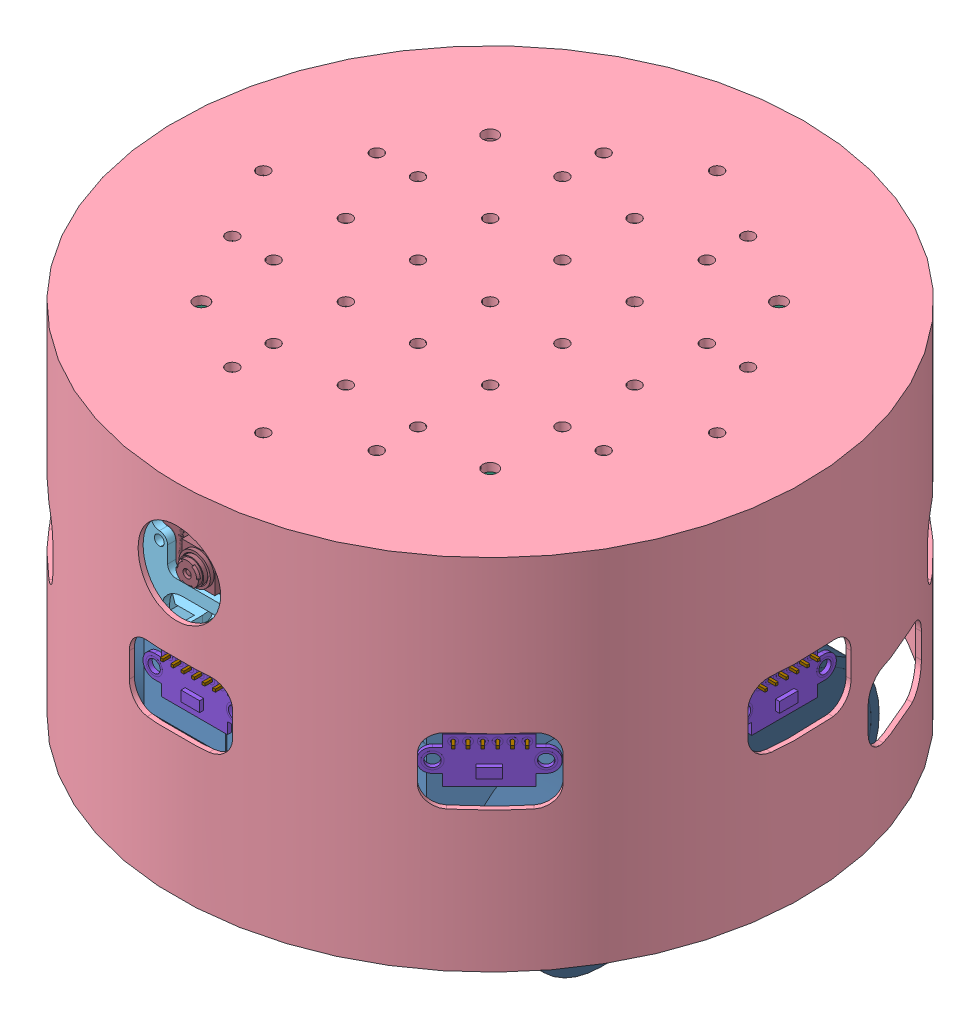
SolidWorks assembly affective_mobile_platform_ver_3, configuration Default. Lengths in mm. (continued)
Components (placement in the parent): (continued)
- outside_case-1: outside_case [Default] at (56.0336 131.8592 98.8354) size (152 87 152)
- 12x1_male_header_pin_AP203-2: 12x1_male_header_pin_AP203 [Default] at (105.1021 111.9373 83.4854) size (2.53 11.54 50.8)
  - 12x1_male_header_pin_AP203.STEP-3: 12x1_male_header_pin_AP203.STEP [Default] at origin size (2.53 11.54 30.48)
    - pin_Predeterminado.STEP-1: pin_Predeterminado.STEP [Default] at (-1.1265 -5.218 11.222) size (0.64 11.54 0.64)
    - pin_body_Predeterminado.STEP-1: pin_body_Predeterminado.STEP [Default] at (-2.0646 3.322 12.8973) x (1 0 0) z (0 -1 0) size (2.53 30.48 2.54)
    - pin_Predeterminado.STEP-2: pin_Predeterminado.STEP [Default] at (-1.1265 -5.218 13.762) size (0.64 11.54 0.64)
    - pin_Predeterminado.STEP-3: pin_Predeterminado.STEP [Default] at (-1.1265 -5.218 16.302) size (0.64 11.54 0.64)
    - pin_Predeterminado.STEP-4: pin_Predeterminado.STEP [Default] at (-1.1265 -5.218 18.842) size (0.64 11.54 0.64)
    - pin_Predeterminado.STEP-5: pin_Predeterminado.STEP [Default] at (-1.1265 -5.218 21.382) size (0.64 11.54 0.64)
    - pin_Predeterminado.STEP-6: pin_Predeterminado.STEP [Default] at (-1.1265 -5.218 23.922) size (0.64 11.54 0.64)
    - pin_Predeterminado.STEP-7: pin_Predeterminado.STEP [Default] at (-1.1265 -5.218 26.462) size (0.64 11.54 0.64)
    - pin_Predeterminado.STEP-8: pin_Predeterminado.STEP [Default] at (-1.1265 -5.218 29.002) size (0.64 11.54 0.64)
    - pin_Predeterminado.STEP-9: pin_Predeterminado.STEP [Default] at (-1.1265 -5.218 31.542) size (0.64 11.54 0.64)
    - pin_Predeterminado.STEP-10: pin_Predeterminado.STEP [Default] at (-1.1265 -5.218 34.082) size (0.64 11.54 0.64)
    - pin_Predeterminado.STEP-11: pin_Predeterminado.STEP [Default] at (-1.1265 -5.218 36.622) size (0.64 11.54 0.64)
    - pin_Predeterminado.STEP-12: pin_Predeterminado.STEP [Default] at (-1.1265 -5.218 39.162) size (0.64 11.54 0.64)
  - 12x1_male_header_pin_AP203.STEP-2: 12x1_male_header_pin_AP203.STEP [Default] at (0 0 -20.32) size (2.53 11.54 30.48)
    - pin_Predeterminado.STEP-1: pin_Predeterminado.STEP [Default] at (-1.1265 -5.218 11.222) size (0.64 11.54 0.64)
    - pin_body_Predeterminado.STEP-1: pin_body_Predeterminado.STEP [Default] at (-2.0646 3.322 12.8973) x (1 0 0) z (0 -1 0) size (2.53 30.48 2.54)
    - pin_Predeterminado.STEP-2: pin_Predeterminado.STEP [Default] at (-1.1265 -5.218 13.762) size (0.64 11.54 0.64)
    - pin_Predeterminado.STEP-3: pin_Predeterminado.STEP [Default] at (-1.1265 -5.218 16.302) size (0.64 11.54 0.64)
    - pin_Predeterminado.STEP-4: pin_Predeterminado.STEP [Default] at (-1.1265 -5.218 18.842) size (0.64 11.54 0.64)
    - pin_Predeterminado.STEP-5: pin_Predeterminado.STEP [Default] at (-1.1265 -5.218 21.382) size (0.64 11.54 0.64)
    - pin_Predeterminado.STEP-6: pin_Predeterminado.STEP [Default] at (-1.1265 -5.218 23.922) size (0.64 11.54 0.64)
    - pin_Predeterminado.STEP-7: pin_Predeterminado.STEP [Default] at (-1.1265 -5.218 26.462) size (0.64 11.54 0.64)
    - pin_Predeterminado.STEP-8: pin_Predeterminado.STEP [Default] at (-1.1265 -5.218 29.002) size (0.64 11.54 0.64)
    - pin_Predeterminado.STEP-9: pin_Predeterminado.STEP [Default] at (-1.1265 -5.218 31.542) size (0.64 11.54 0.64)
    - pin_Predeterminado.STEP-10: pin_Predeterminado.STEP [Default] at (-1.1265 -5.218 34.082) size (0.64 11.54 0.64)
    - pin_Predeterminado.STEP-11: pin_Predeterminado.STEP [Default] at (-1.1265 -5.218 36.622) size (0.64 11.54 0.64)
    - pin_Predeterminado.STEP-12: pin_Predeterminado.STEP [Default] at (-1.1265 -5.218 39.162) size (0.64 11.54 0.64)
- 13x2_female_header^affective_mobile_platform_ver_3-2: 13x2_female_header^affective_mobile_platform_ver_3 [Default] at (128.2122 91.0473 108.7584) x (0 0 1) z (0 1 0) size (50.8 2.5 18) (virtual)
  - Body_Varsay_lan.STEP^13x2_female_header_affective_mobile_platform_ver_3-2: Body_Varsay_lan.STEP^13x2_female_header_affective_mobile_platform_ver_3 [Default] at (33.296 -42.1751 13.1719) size (33.02 2.5 8.5) (virtual)
  - pin_Varsay_lan.STEP^13x2_female_header_affective_mobile_platform_ver_3-28: pin_Varsay_lan.STEP^13x2_female_header_affective_mobile_platform_ver_3 [Default] at (22.3287 -23.5891 -26.7452) x (1 0 0) z (0 -1 0) size (2 16.29 0.4) (virtual)
  - pin_Varsay_lan.STEP^13x2_female_header_affective_mobile_platform_ver_3-30: pin_Varsay_lan.STEP^13x2_female_header_affective_mobile_platform_ver_3 [Default] at (24.8687 -23.5891 -26.7452) x (1 0 0) z (0 -1 0) size (2 16.29 0.4) (virtual)
  - pin_Varsay_lan.STEP^13x2_female_header_affective_mobile_platform_ver_3-32: pin_Varsay_lan.STEP^13x2_female_header_affective_mobile_platform_ver_3 [Default] at (27.4087 -23.5891 -26.7452) x (1 0 0) z (0 -1 0) size (2 16.29 0.4) (virtual)
  - pin_Varsay_lan.STEP^13x2_female_header_affective_mobile_platform_ver_3-34: pin_Varsay_lan.STEP^13x2_female_header_affective_mobile_platform_ver_3 [Default] at (29.9487 -23.5891 -26.7452) x (1 0 0) z (0 -1 0) size (2 16.29 0.4) (virtual)
  - pin_Varsay_lan.STEP^13x2_female_header_affective_mobile_platform_ver_3-36: pin_Varsay_lan.STEP^13x2_female_header_affective_mobile_platform_ver_3 [Default] at (32.4887 -23.5891 -26.7452) x (1 0 0) z (0 -1 0) size (2 16.29 0.4) (virtual)
  - pin_Varsay_lan.STEP^13x2_female_header_affective_mobile_platform_ver_3-38: pin_Varsay_lan.STEP^13x2_female_header_affective_mobile_platform_ver_3 [Default] at (35.0287 -23.5891 -26.7452) x (1 0 0) z (0 -1 0) size (2 16.29 0.4) (virtual)
  - pin_Varsay_lan.STEP^13x2_female_header_affective_mobile_platform_ver_3-40: pin_Varsay_lan.STEP^13x2_female_header_affective_mobile_platform_ver_3 [Default] at (37.5687 -23.5891 -26.7452) x (1 0 0) z (0 -1 0) size (2 16.29 0.4) (virtual)
  - pin_Varsay_lan.STEP^13x2_female_header_affective_mobile_platform_ver_3-42: pin_Varsay_lan.STEP^13x2_female_header_affective_mobile_platform_ver_3 [Default] at (40.1087 -23.5891 -26.7452) x (1 0 0) z (0 -1 0) size (2 16.29 0.4) (virtual)
  - pin_Varsay_lan.STEP^13x2_female_header_affective_mobile_platform_ver_3-44: pin_Varsay_lan.STEP^13x2_female_header_affective_mobile_platform_ver_3 [Default] at (42.6487 -23.5891 -26.7452) x (1 0 0) z (0 -1 0) size (2 16.29 0.4) (virtual)
  - pin_Varsay_lan.STEP^13x2_female_header_affective_mobile_platform_ver_3-46: pin_Varsay_lan.STEP^13x2_female_header_affective_mobile_platform_ver_3 [Default] at (45.1887 -23.5891 -26.7452) x (1 0 0) z (0 -1 0) size (2 16.29 0.4) (virtual)
  - pin_Varsay_lan.STEP^13x2_female_header_affective_mobile_platform_ver_3-48: pin_Varsay_lan.STEP^13x2_female_header_affective_mobile_platform_ver_3 [Default] at (47.7287 -23.5891 -26.7452) x (1 0 0) z (0 -1 0) size (2 16.29 0.4) (virtual)
  - pin_Varsay_lan.STEP^13x2_female_header_affective_mobile_platform_ver_3-50: pin_Varsay_lan.STEP^13x2_female_header_affective_mobile_platform_ver_3 [Default] at (50.2687 -23.5891 -26.7452) x (1 0 0) z (0 -1 0) size (2 16.29 0.4) (virtual)
  - pin_Varsay_lan.STEP^13x2_female_header_affective_mobile_platform_ver_3-52: pin_Varsay_lan.STEP^13x2_female_header_affective_mobile_platform_ver_3 [Default] at (52.8087 -23.5891 -26.7452) x (1 0 0) z (0 -1 0) size (2 16.29 0.4) (virtual)
  - Body_Varsay_lan.STEP^13x2_female_header_affective_mobile_platform_ver_3-3: Body_Varsay_lan.STEP^13x2_female_header_affective_mobile_platform_ver_3 [Default] at (51.076 -42.1751 13.1719) size (33.02 2.5 8.5) (virtual)
  - pin_Varsay_lan.STEP^13x2_female_header_affective_mobile_platform_ver_3-53: pin_Varsay_lan.STEP^13x2_female_header_affective_mobile_platform_ver_3 [Default] at (55.3487 -23.5891 -26.7452) x (1 0 0) z (0 -1 0) size (2 16.29 0.4) (virtual)
  - pin_Varsay_lan.STEP^13x2_female_header_affective_mobile_platform_ver_3-54: pin_Varsay_lan.STEP^13x2_female_header_affective_mobile_platform_ver_3 [Default] at (57.8887 -23.5891 -26.7452) x (1 0 0) z (0 -1 0) size (2 16.29 0.4) (virtual)
  - pin_Varsay_lan.STEP^13x2_female_header_affective_mobile_platform_ver_3-55: pin_Varsay_lan.STEP^13x2_female_header_affective_mobile_platform_ver_3 [Default] at (60.4287 -23.5891 -26.7452) x (1 0 0) z (0 -1 0) size (2 16.29 0.4) (virtual)
  - pin_Varsay_lan.STEP^13x2_female_header_affective_mobile_platform_ver_3-56: pin_Varsay_lan.STEP^13x2_female_header_affective_mobile_platform_ver_3 [Default] at (62.9687 -23.5891 -26.7452) x (1 0 0) z (0 -1 0) size (2 16.29 0.4) (virtual)
  - pin_Varsay_lan.STEP^13x2_female_header_affective_mobile_platform_ver_3-57: pin_Varsay_lan.STEP^13x2_female_header_affective_mobile_platform_ver_3 [Default] at (70.5887 -23.5891 -26.7452) x (1 0 0) z (0 -1 0) size (2 16.29 0.4) (virtual)
  - pin_Varsay_lan.STEP^13x2_female_header_affective_mobile_platform_ver_3-58: pin_Varsay_lan.STEP^13x2_female_header_affective_mobile_platform_ver_3 [Default] at (68.0487 -23.5891 -26.7452) x (1 0 0) z (0 -1 0) size (2 16.29 0.4) (virtual)
  - pin_Varsay_lan.STEP^13x2_female_header_affective_mobile_platform_ver_3-61: pin_Varsay_lan.STEP^13x2_female_header_affective_mobile_platform_ver_3 [Default] at (65.5087 -23.5891 -26.7452) x (1 0 0) z (0 -1 0) size (2 16.29 0.4) (virtual)
- pi_cam_holder-1: pi_cam_holder [Default] at (56.0336 90.9064 152.5354) size (63.18 39 21.14)
Mates (geometry in assembly coordinates):
- Coincident1: coincident anti-aligned: plane of main_case_v02-1 through (23.7836 61.1064 146.5354) normal (0 1 0); plane of power_bank-1 through (23.7836 62.6064 146.5354) normal (0 -1 0)
- Coincident2: coincident anti-aligned: plane of main_case-1 through (56.0336 74.2064 146.5354) normal (0 0 -1); plane of power_bank-1 through (56.0336 74.1064 146.5354) normal (0 0 1)
- Width1: width aligned: plane of power_bank-1 through (23.7836 62.6064 146.5354) normal (-1 0 0); plane of power_bank-1 through (88.2836 62.6064 146.5354) normal (1 0 0); plane of main_case-1 through (88.2836 59.1064 146.5354) normal (-1 0 0); plane of main_case-1 through (23.7836 89.3064 146.5354) normal (1 0 0)
- Coincident9: coincident anti-aligned: plane of main_case-1 through (56.0336 74.2064 74.8354) normal (0 0 1); plane of motor_holder-1 through (56.0336 51.1064 74.8354) normal (0 0 -1)
- Coincident10: coincident anti-aligned: plane of main_case-1 through (56.0336 74.2064 51.1354) normal (1 0 0); plane of motor_holder-1 through (56.0336 51.1064 74.8354) normal (-1 0 0)
- Coincident17: coincident aligned: plane of main_case-1 through (94.0836 56.1064 115.3354) normal (1 0 0); plane of wheel_holder-1 through (94.0836 50.1064 122.8354) normal (1 0 0)
- Coincident18: coincident aligned: plane of main_case-1 through (56.0336 74.2064 122.8354) normal (0 0 1); plane of wheel_holder-1 through (74.0836 50.1064 122.8354) normal (0 0 1)
- Concentric1: concentric anti-aligned: cylinder of main_case-1 through (29.5836 56.1064 112.3354) axis (0 -1 0) radius 1.6; cylinder of wheel_holder-2 through (29.5836 51.1064 112.3354) axis (0 1 0) radius 1.6
- Concentric2: concentric anti-aligned: cylinder of main_case-1 through (29.5836 56.1064 133.3354) axis (0 -1 0) radius 1.6; cylinder of wheel_holder-2 through (29.5836 51.1064 133.3354) axis (0 1 0) radius 1.6
- Coincident21: coincident anti-aligned: plane of main_case-1 through (56.0336 56.1064 51.1354) normal (0 -1 0); plane of wheel_holder-1 through (94.0836 56.1064 130.3354) normal (0 1 0)
- Coincident22: coincident anti-aligned: plane of main_case-1 through (56.0336 56.1064 51.1354) normal (0 -1 0); plane of wheel_holder-2 through (17.9836 56.1064 115.3354) normal (0 1 0)
- Coincident23: coincident anti-aligned: plane of main_case-1 through (56.0336 56.1064 51.1354) normal (0 -1 0); plane of motor_holder-1 through (21.7836 56.1064 82.8354) normal (0 1 0)
- Width2: width anti-aligned: plane of power_bank-2 through (56.0336 72.6064 51.0354) normal (0 0 -1); plane of main_case-1 through (56.0336 72.6064 146.6354) normal (0 0 1); plane of power_bank-2 through (56.0336 74.2064 51.1354) normal (0 0 1); plane of main_case-1 through (56.0336 74.2064 146.5354) normal (0 0 -1)
- Width3: width aligned: plane of power_bank-2 through (23.7836 61.1064 51.0354) normal (-1 0 0); plane of main_case-1 through (88.2836 61.1064 51.0354) normal (1 0 0); plane of power_bank-2 through (88.2836 59.1064 146.5354) normal (-1 0 0); plane of main_case-1 through (23.7836 89.3064 146.5354) normal (1 0 0)
- InPlace1: in place: plane of main_case-1 through (21.7836 85.8064 146.5354) normal (0 1 0); plane of ? through (0 85.8064 0) normal (0 1 0); moOrthogonalPlaneRef_w of main_case-1 through (21.7836 85.8064 146.5354) normal (0 1 0); plane of ? through (0 85.8064 0) normal (0 0 -1); plane of main_case-1 through (21.7836 85.8064 146.5354) normal (0 1 0); plane of ? through (0 85.8064 0) normal (1 0 0); plane of main_case-1 through (21.7836 89.3064 146.5354) normal (0 1 0); unknown of ?
- Coincident25: coincident aligned: plane of main_case-1; plane of ?
- Coincident26: coincident aligned: moOrthogonalPlaneRef_w of main_case-1 through (56.0336 89.3064 51.1354) normal (0 0 -1); plane of case_cap-1 through (56.0336 85.8064 51.1354) normal (0 0 -1)
- Coincident27: coincident anti-aligned: moOrthogonalPlaneRef_w of main_case-1 through (56.0336 89.3064 51.1354) normal (-1 0 0); plane of case_cap-1 through (56.0336 85.8064 51.1354) normal (1 0 0)
- Distance1: distance = 3 mm anti-aligned: plane of Raspberry Pi 3 Light Version-1 through (28.0336 94.6664 56.3733) normal (0 -1 0); plane of case_cap-1 through (29.5836 87.8064 152.5354) normal (0 1 0)
- Coincident41: coincident aligned: plane of main_case-1 through (56.0336 74.2064 51.1354) normal (1 0 0); plane of 2nd_layer-1 through (56.0336 89.3064 98.8354) normal (1 0 0)
- Coincident46: coincident: plane of 2nd_layer-1 through (56.0336 90.9064 98.8354) normal (0 1 0); plane of H254_90deg_3pin-1/FrameAndPin_H254_90deg-2/frame_H254-1 through (53.4936 109.8864 47.2354) normal (0 -1 0)
- Coincident47: coincident: plane of 2nd_layer-1 through (56.0336 89.3064 98.8354) normal (1 0 0); line of H254_90deg_3pin-1/FrameAndPin_H254_90deg-2/frame_H254-1 through (56.0336 112.4264 47.2354) axis (0 0 -1)
- Coincident50: coincident: plane of 2nd_layer-1 through (56.0336 90.9064 98.8354) normal (0 1 0); line of H254_90deg_3pin-1/FrameAndPin_H254_90deg-2/frame_H254-1 through (53.4936 109.8864 38.8354) axis (1 0 0)
- Tangent3: tangent aligned: cylinder of 2nd_layer-1 through (56.0336 90.9064 98.8354) axis (0 -1 0) radius 65; plane of H254_90deg_3pin-1/FrameAndPin_H254_90deg-2/frame_H254-1 through (53.4936 112.4264 38.8354) normal (0 0 -1)
- Coincident55: coincident aligned: plane of main_case-1 through (56.0336 74.2064 98.8354) normal (0 0 1); plane of 2nd_layer-1 through (56.0336 89.3064 98.8354) normal (0 0 1)
- Coincident62: coincident aligned: plane of motor_holder-1 through (96.4836 51.1064 74.8354) normal (1 0 0); circle of wheels-1
- Parallel3: parallel aligned: plane of main_case-1 through (56.0336 58.1064 51.1354) normal (0 1 0); plane of wheels-1 through (106.8336 70.6064 122.8354) normal (0 1 0)
- Concentric3: concentric aligned: cylinder of wheel_holder-1 through (84.0836 51.1064 122.8354) axis (1 0 0) radius 1.6; circle of wheels-1
- Coincident64: coincident aligned: plane of wheels-1 through (106.8336 70.6064 122.8354) normal (0 1 0); plane of wheels-2 through (5.2336 70.6064 74.8354) normal (0 1 0)
- Coincident65: coincident anti-aligned: plane of main_case-1 through (15.5836 58.1064 82.8354) normal (-1 0 0); plane of wheels-2 through (15.5836 51.1064 74.8354) normal (1 0 0)
- Concentric4: concentric anti-aligned: cylinder of wheel_holder-2 through (17.9836 51.1064 122.8354) axis (1 0 0) radius 1.8; circle of wheels-2
- Coincident70: coincident anti-aligned: plane of main_case-1 through (21.7836 89.3064 146.5354) normal (0 1 0); plane of 2nd_layer-1 through (56.0336 89.3064 98.8354) normal (0 -1 0)
- Coincident73: coincident anti-aligned: plane of Raspberry Pi 3 Light Version-1 through (34.0436 98.4964 134.2075) normal (0 1 0); plane of Buchsenleiste 2X15-3/Buchsenleiste-1 through (30.2636 98.4964 132.9275) normal (0 -1 0)
- Width12: width anti-aligned: plane of Buchsenleiste 2X15-3/Buchsenleiste-1 through (99.2987 106.1664 123.3705) normal (-0.866025 0 0.5); plane of Buchsenleiste 2X15-3/Buchsenleiste-16 through (103.6981 106.1664 120.8305) normal (0.866025 0 -0.5); plane of Raspberry Pi 3 Light Version-1 through (34.0336 95.9864 133.6789) normal (1 0 0); plane of Raspberry Pi 3 Light Version-1 through (29.0336 95.9864 132.176) normal (-1 0 0)
- Coincident75: coincident aligned: plane of Raspberry Pi 3 Light Version-1 through (30.1676 95.9864 134.1975) normal (0 0 1); plane of Buchsenleiste 2X15-3/Buchsenleiste-1 through (28.9936 98.4964 134.1975) normal (0 0 1)
- InPlace2: in place: plane of ? through (81.8036 107.9964 64.7433) normal (0 1 0); plane of ? through (0 107.9964 0) normal (0 1 0); plane of ? through (81.8036 107.9964 64.7433) normal (0 1 0); plane of ? through (0 107.9964 0) normal (0 0 -1); plane of ? through (81.8036 107.9964 64.7433) normal (0 1 0); plane of ? through (0 107.9964 0) normal (1 0 0); plane of ? through (101.0336 114.6664 123.8354) normal (0 1 0); unknown of ?
- Coincident76: coincident aligned: plane of ?; plane of ?
- Coincident77: coincident aligned: moOrthogonalPlaneRef_w of Buchsenleiste 2X15-3/Buchsenleiste-1; plane of Part4^affective_mobile_platform_ver_3-1 through (101.0336 114.6664 123.8354) normal (0.866025 0 -0.5)
- Coincident78: coincident anti-aligned: moOrthogonalPlaneRef_w of Buchsenleiste 2X15-3/Buchsenleiste-1 through (101.0336 114.6664 123.8354) axis (-0.5 0 -0.866025); plane of Part4^affective_mobile_platform_ver_3-1 through (101.0336 114.6664 123.8354) normal (0.5 0 0.866025)
- Concentric5: concentric aligned: cylinder of 2nd_layer-1 through (80.5336 89.3064 137.7975) axis (0 1 0) radius 1.2; cylinder of spacer-1 through (31.5336 83.6664 59.8733) axis (0 1 0) radius 0.98
- Coincident79: coincident anti-aligned: plane of 2nd_layer-1 through (56.0336 90.9064 98.8354) normal (0 1 0); plane of spacer-1 through (31.5336 89.6664 59.8733) normal (0 -1 0)
- Parallel4: parallel aligned: plane of main_case-1 through (21.7836 56.1064 49.1354) normal (0 0 -1); plane of spacer-1 through (32.7171 94.6664 57.8233) normal (0 0 -1)
- Coincident81: coincident anti-aligned: plane of 2nd_layer-1 through (56.0336 90.9064 98.8354) normal (0 1 0); plane of spacer-2 through (31.5336 90.9064 137.7975) normal (0 -1 0)
- Coincident82: coincident aligned: plane of spacer-1 through (32.7171 94.6664 57.8233) normal (0 0 -1); plane of spacer-2 through (29.2525 105.9064 134.9643) normal (-0.932571 0 -0.360988)
- Coincident85: coincident anti-aligned: plane of 2nd_layer-1 through (56.0336 90.9064 98.8354) normal (0 1 0); plane of spacer-4 through (80.5336 90.9064 79.7975) normal (0 -1 0)
- Parallel5: parallel anti-aligned: plane of spacer-1 through (30.35 94.6664 61.9233) normal (0 0 1); plane of spacer-4 through (78.7149 105.9064 82.9475) normal (0 0 1)
- Coincident88: coincident anti-aligned: plane of 2nd_layer-1 through (56.0336 90.9064 98.8354) normal (0 1 0); plane of spacer-5 through (31.5336 90.9064 79.7975) normal (0 -1 0)
- Coincident89: coincident aligned: plane of spacer-4 through (82.3522 105.9064 76.6475) normal (0 0 -1); plane of spacer-5 through (33.3522 105.9064 76.6475) normal (0 0 -1)
- Coincident90: coincident anti-aligned: plane of Raspberry Pi 3 Light Version-1 through (28.0336 94.6664 56.3733) normal (0 -1 0); plane of spacer-5 through (31.5336 105.9064 79.7975) normal (0 1 0)
- InPlace3: in place: plane of ? through (29.5836 53.1064 112.3354) normal (0 -1 0); plane of ? through (0 53.1064 0) normal (0 -1 0); plane of ? through (29.5836 53.1064 112.3354) normal (0 -1 0); plane of ? through (0 53.1064 0) normal (0 0 -1); plane of ? through (29.5836 53.1064 112.3354) normal (0 -1 0); plane of ? through (0 53.1064 0) normal (-1 0 0); plane of wheel_holder-2 through (29.5836 51.1064 112.3354) normal (0 -1 0); unknown of 1st_layer-1
- Coincident91: coincident aligned: plane of wheel_holder-2; plane of 1st_layer-1
- Coincident92: coincident aligned: moOrthogonalPlaneRef_w of wheel_holder-2 through (37.9836 51.1064 122.8354) normal (-1 0 0); plane of 1st_layer-1 through (37.9836 51.1064 122.8354) normal (-1 0 0)
- Coincident93: coincident anti-aligned: moOrthogonalPlaneRef_w of wheel_holder-2 through (37.9836 51.1064 122.8354) normal (0 0 -1); plane of 1st_layer-1 through (37.9836 51.1064 122.8354) normal (0 0 1)
- Concentric10: concentric aligned: cylinder of main_case-1 through (35.2836 59.1064 138.5354) axis (0 -1 0) radius 1.6; cylinder of spacer-7 through (35.2836 62.1064 138.5354) axis (0 -1 0) radius 1.5
- Coincident95: coincident anti-aligned: plane of main_case-1 through (56.0336 56.1064 51.1354) normal (0 -1 0); plane of spacer-7 through (35.2836 56.1064 138.5354) normal (0 1 0)
- Concentric11: concentric aligned: cylinder of 2nd_layer-1 through (101.0336 89.3064 118.8354) axis (0 1 0) radius 1.6; cylinder of M3_spacer-1 through (101.0336 84.9064 118.8354) axis (0 1 0) radius 1.5
- Coincident96: coincident anti-aligned: plane of 2nd_layer-1 through (56.0336 90.9064 98.8354) normal (0 1 0); plane of M3_spacer-1 through (101.0336 90.9064 118.8354) normal (0 -1 0)
- Parallel6: parallel aligned: plane of main_case-1 through (90.2836 56.1064 49.1354) normal (1 0 0); plane of M3_spacer-1 through (104.0336 115.9064 120.5674) normal (1 0 0)
- Concentric12: concentric aligned: circle of pcb_sensor_led-1; cylinder of M3_spacer-2 through (101.0336 84.9064 78.8354) axis (0 1 0) radius 1.5
- Coincident98: coincident anti-aligned: plane of 2nd_layer-1 through (56.0336 90.9064 98.8354) normal (0 1 0); plane of M3_spacer-2 through (101.0336 90.9064 78.8354) normal (0 -1 0)
- Concentric13: concentric aligned: cylinder of 2nd_layer-1 through (11.0336 89.3064 78.8354) axis (0 1 0) radius 1.6; cylinder of M3_spacer-3 through (11.0336 84.9064 78.8354) axis (0 1 0) radius 1.5
- Coincident100: coincident anti-aligned: plane of 2nd_layer-1 through (56.0336 90.9064 98.8354) normal (0 1 0); plane of M3_spacer-3 through (11.0336 90.9064 78.8354) normal (0 -1 0)
- Concentric14: concentric aligned: cylinder of 2nd_layer-1 through (11.0336 89.3064 118.8354) axis (0 1 0) radius 1.6; cylinder of M3_spacer-4 through (11.0336 84.9064 118.8354) axis (0 1 0) radius 1.5
- Coincident102: coincident anti-aligned: plane of 2nd_layer-1 through (56.0336 90.9064 98.8354) normal (0 1 0); plane of M3_spacer-4 through (11.0336 90.9064 118.8354) normal (0 -1 0)
- InPlace5: in place: plane of ? through (101.0336 114.6664 68.8354) normal (0 1 0); plane of ? through (0 114.6664 0) normal (0 1 0); plane of ? through (101.0336 114.6664 68.8354) normal (0 1 0); plane of ? through (0 114.6664 0) normal (0 0 -1); plane of ? through (101.0336 114.6664 68.8354) normal (0 1 0); plane of ? through (0 114.6664 0) normal (1 0 0); plane of ? through (101.0336 115.9064 78.8354) normal (0 1 0); unknown of assembly
- Coincident107: coincident: plane of ?; plane of ?
- Coincident108: coincident: moOrthogonalPlaneRef_w of M3_spacer-2; plane of Part9^affective_mobile_platform_ver_3-1 through (0 0 0) normal (0 1 0)
- Coincident109: coincident: moOrthogonalPlaneRef_w of M3_spacer-2; plane of Part9^affective_mobile_platform_ver_3-1 through (0 0 0) normal (1 0 0)
- Parallel8: parallel aligned: plane of main_case-1 through (90.2836 56.1064 49.1354) normal (1 0 0); plane of M3_spacer-2 through (104.0336 115.9064 80.5674) normal (1 0 0)
- InPlace6: in place: plane of ? through (101.0336 114.6664 68.8354) normal (0 1 0); plane of ? through (0 114.6664 0) normal (0 1 0); plane of ? through (101.0336 114.6664 68.8354) normal (0 1 0); plane of ? through (0 114.6664 0) normal (0 0 -1); plane of ? through (101.0336 114.6664 68.8354) normal (0 1 0); plane of ? through (0 114.6664 0) normal (1 0 0); plane of ? through (101.0336 115.9064 78.8354) normal (0 1 0); unknown of ?
- Coincident111: coincident aligned: plane of ?; plane of ?
- Coincident112: coincident aligned: moOrthogonalPlaneRef_w of M3_spacer-2 through (101.0336 115.9064 78.8354) normal (0.866025 0 0.5); plane of Part10^affective_mobile_platform_ver_3-1 through (101.0336 114.6664 68.8354) normal (0.866025 0 0.5)
- Coincident113: coincident anti-aligned: moOrthogonalPlaneRef_w of M3_spacer-2 through (101.0336 115.9064 78.8354) normal (0.5 0 -0.866025); plane of Part10^affective_mobile_platform_ver_3-1 through (101.0336 114.6664 68.8354) normal (-0.5 0 0.866025)
- Width14: width anti-aligned: plane of Raspberry Pi 3 Light Version-1 through (84.0336 94.2364 138.3075) normal (1 0 0); plane of main_case-1 through (28.0336 94.2364 59.3633) normal (-1 0 0); plane of Raspberry Pi 3 Light Version-1 through (21.7836 56.1064 148.5354) normal (-1 0 0); plane of main_case-1 through (90.2836 56.1064 49.1354) normal (1 0 0)
- Width15: width anti-aligned: plane of Raspberry Pi 3 Light Version-1 through (81.0436 94.2364 56.3733) normal (0 0 -1); plane of main_case-1 through (31.0236 94.2364 141.2975) normal (0 0 1); plane of Raspberry Pi 3 Light Version-1 through (90.2836 56.1064 148.5354) normal (0 0 1); plane of main_case-1 through (21.7836 56.1064 49.1354) normal (0 0 -1)
- Coincident120: coincident anti-aligned: plane of 2nd_layer-1 through (56.0336 90.9064 98.8354) normal (0 1 0); plane of 874381243-2 through (56.0336 90.6664 232.6926) normal (0 -1 0)
- Width17: width anti-aligned: plane of 874381243-2 through (46.3836 95.1164 235.5676) normal (-1 0 0); plane of 874381243-2 through (65.6836 95.1164 229.8176) normal (1 0 0); plane of 2nd_layer-1 through (47.3086 88.5464 163.3354) normal (-1 0 0); plane of 2nd_layer-1 through (64.7586 88.5464 163.3354) normal (1 0 0)
- InPlace7: in place: plane of ? through (11.0336 114.6664 73.8354) normal (0 1 0); plane of ? through (0 114.6664 0) normal (0 1 0); plane of ? through (11.0336 114.6664 73.8354) normal (0 1 0); plane of ? through (0 114.6664 0) normal (0 0 -1); plane of ? through (11.0336 114.6664 73.8354) normal (0 1 0); plane of ? through (0 114.6664 0) normal (1 0 0); plane of ? through (11.0336 115.9064 78.8354) normal (0 1 0); unknown of 3rd_layer-1
- Coincident124: coincident aligned: plane of ?; plane of 3rd_layer-1
- Coincident125: coincident aligned: moOrthogonalPlaneRef_w of M3_spacer-3; plane of 3rd_layer-1 through (56.0336 115.2592 98.8354) normal (0 0 1)
- Coincident126: coincident anti-aligned: moOrthogonalPlaneRef_w of M3_spacer-3; plane of 3rd_layer-1 through (56.0336 115.2592 98.8354) normal (-1 0 0)
- InPlace8: in place: plane of ? through (11.0336 114.6664 123.8354) normal (0 1 0); plane of ? through (0 114.6664 0) normal (0 1 0); plane of ? through (11.0336 114.6664 123.8354) normal (0 1 0); plane of ? through (0 114.6664 0) normal (0 0 -1); plane of ? through (11.0336 114.6664 123.8354) normal (0 1 0); plane of ? through (0 114.6664 0) normal (1 0 0); plane of ? through (11.0336 115.9064 118.8354) normal (0 1 0); unknown of ?
- Coincident127: coincident aligned: plane of ?; plane of ?
- Coincident128: coincident aligned: moOrthogonalPlaneRef_w of M3_spacer-4 through (11.0336 115.9064 118.8354) normal (0.866025 0 0.5); plane of Part2^affective_mobile_platform_ver_3-1 through (11.0336 114.6664 123.8354) normal (0.866025 0 0.5)
- Coincident129: coincident anti-aligned: moOrthogonalPlaneRef_w of M3_spacer-4 through (11.0336 115.9064 118.8354) normal (0.5 0 -0.866025); plane of Part2^affective_mobile_platform_ver_3-1 through (11.0336 114.6664 123.8354) normal (-0.5 0 0.866025)
- InPlace9: in place: plane of ? through (101.0336 114.6664 123.8354) normal (0 1 0); plane of ? through (0 114.6664 0) normal (0 1 0); plane of ? through (101.0336 114.6664 123.8354) normal (0 1 0); plane of ? through (0 114.6664 0) normal (0 0 -1); plane of ? through (101.0336 114.6664 123.8354) normal (0 1 0); plane of ? through (0 114.6664 0) normal (1 0 0); plane of ? through (101.0336 115.9064 118.8354) normal (0 1 0); unknown of ?
- Coincident130: coincident aligned: plane of ?; plane of ?
- Coincident131: coincident aligned: moOrthogonalPlaneRef_w of M3_spacer-1 through (101.0336 115.9064 118.8354) normal (0.866025 0 -0.5); plane of Part4^affective_mobile_platform_ver_3-1 through (101.0336 114.6664 123.8354) normal (0.866025 0 -0.5)
- Coincident132: coincident anti-aligned: moOrthogonalPlaneRef_w of M3_spacer-1 through (101.0336 115.9064 118.8354) normal (-0.5 0 -0.866025); plane of Part4^affective_mobile_platform_ver_3-1 through (101.0336 114.6664 123.8354) normal (0.5 0 0.866025)
- Parallel12: parallel aligned: plane of spacer-2 through (33.8146 105.9064 140.6306) normal (0.932571 0 0.360988); plane of spacer-8 through (82.8146 105.9064 140.6306) normal (0.932571 0 0.360988)
- Coincident134: coincident aligned: plane of spacer-2 through (31.5336 105.9064 137.7975) normal (0 1 0); plane of spacer-8 through (80.5336 105.9064 137.7975) normal (0 1 0)
- Width19: width: plane of Buchsenleiste 2X15-3/Buchsenleiste-39 through (28.9936 98.4664 85.1675) normal (0 0 -1); plane of Buchsenleiste 2X15-3/Buchsenleiste-39 through (28.9936 98.4664 84.1675) normal (0 0 1); plane of raspberryPi3B-1 through (82.0536 97.4064 84.4175) normal (0 0 -1); plane of raspberryPi3B-1 through (82.0536 97.4064 84.9175) normal (0 0 1)
- Width20: width: plane of Buchsenleiste 2X15-3/Buchsenleiste-39 through (29.7636 98.4664 83.3975) normal (1 0 0); plane of Buchsenleiste 2X15-3/Buchsenleiste-39 through (30.7636 98.4664 83.3975) normal (-1 0 0); plane of raspberryPi3B-1 through (82.0536 97.4064 84.9175) normal (1 0 0); plane of raspberryPi3B-1 through (81.5536 97.4064 84.9175) normal (-1 0 0)
- Coincident135: coincident anti-aligned: plane of Buchsenleiste 2X15-3/Buchsenleiste-39 through (30.2636 98.4664 84.6675) normal (0 -1 0); plane of raspberryPi3B-1 through (56.0336 103.4064 98.7975) normal (0 -1 0)
- InPlace10: in place: plane of ? through (0 102.1664 0) normal (0 1 0); plane of ? through (0 102.1664 0) normal (0 0 -1); plane of ? through (0 102.1664 0) normal (1 0 0); unknown of ?
- Coincident138: coincident aligned: 
- Coincident139: coincident aligned: plane of Part6^affective_mobile_platform_ver_3-1 through (0 102.1664 0) normal (0 0 -1)
- Coincident140: coincident anti-aligned: plane of Part6^affective_mobile_platform_ver_3-1 through (0 102.1664 0) normal (1 0 0)
- Coincident138: coincident anti-aligned: plane of main_case-1 through (56.0336 61.1064 51.1354) normal (0 1 0); plane of power_bank-2 through (88.2836 61.1064 51.0354) normal (0 -1 0)
- Coincident140: coincident anti-aligned: plane of 2nd_layer-1 through (56.0336 90.9064 98.8354) normal (0 1 0); plane of raspberryPi3B-1 through (56.0336 90.9064 98.7975) normal (0 -1 0)
- Concentric26: concentric anti-aligned: cylinder of raspberryPi3B-1 through (80.5336 107.2064 137.7975) axis (0 -1 0) radius 1.375; cylinder of spacer-8 through (80.5336 102.9064 137.7975) axis (0 1 0) radius 1.5
- Concentric27: concentric anti-aligned: circle of spacer-2; circle of raspberryPi3B-1
- Parallel13: parallel anti-aligned: plane of main_case-1 through (56.0336 74.2064 51.1354) normal (1 0 0); plane of M3_spacer-3 through (11.0336 90.9064 78.8354) normal (-1 0 0)
- InPlace11: in place: plane of ? through (11.0336 115.6664 73.8354) normal (0 1 0); plane of ? through (0 115.6664 0) normal (0 1 0); plane of ? through (11.0336 115.6664 73.8354) normal (0 1 0); plane of ? through (0 115.6664 0) normal (0 0 -1); plane of ? through (11.0336 115.6664 73.8354) normal (0 1 0); plane of ? through (0 115.6664 0) normal (1 0 0); plane of ? through (11.0336 115.9064 78.8354) normal (0 1 0); unknown of 3rd_layer-1
- Coincident142: coincident aligned: plane of ?; plane of 3rd_layer-1
- Coincident143: coincident aligned: moOrthogonalPlaneRef_w of M3_spacer-3 through (11.0336 115.9064 78.8354) normal (1 0 0); plane of 3rd_layer-1 through (56.0336 115.2592 98.8354) normal (0 0 1)
- Coincident144: coincident anti-aligned: moOrthogonalPlaneRef_w of M3_spacer-3 through (11.0336 115.9064 78.8354) normal (0 0 -1); plane of 3rd_layer-1 through (56.0336 115.2592 98.8354) normal (-1 0 0)
- Concentric28: concentric anti-aligned: cylinder of 3rd_layer-1 through (11.0336 117.5064 78.8354) axis (0 -1 0) radius 1.6; cylinder of spacer-9 through (11.0336 113.0264 78.8354) axis (0 1 0) radius 1.5
- Coincident144: coincident anti-aligned: plane of 3rd_layer-1 through (67.2586 117.5064 46.1354) normal (0 1 0); plane of spacer-9 through (11.0336 119.0264 78.8354) normal (0 -1 0)
- Parallel14: parallel aligned: plane of M3_spacer-3 through (9.3015 115.9064 81.8354) normal (0 0 1); plane of spacer-9 through (9.2149 134.0264 81.9854) normal (0 0 1)
- Concentric29: concentric anti-aligned: cylinder of 3rd_layer-1 through (101.0336 117.5064 78.8354) axis (0 -1 0) radius 1.6; cylinder of spacer-10 through (101.0336 113.0264 78.8354) axis (0 1 0) radius 1.5
- Coincident146: coincident anti-aligned: plane of 3rd_layer-1 through (67.2586 117.5064 46.1354) normal (0 1 0); plane of spacer-10 through (101.0336 119.0264 78.8354) normal (0 -1 0)
- Parallel15: parallel aligned: plane of M3_spacer-2 through (101.0336 115.9064 82.2995) normal (0.5 0 0.866025); plane of spacer-10 through (101.0336 134.0264 82.4727) normal (0.5 0 0.866025)
- Concentric30: concentric aligned: cylinder of 2nd_layer-1 through (80.5336 89.3054 137.7975) axis (0 1 0) radius 1.6; cylinder of spacer-8 through (80.5336 102.9064 137.7975) axis (0 1 0) radius 1.5
- Concentric31: concentric aligned: cylinder of 2nd_layer-1 through (31.5336 89.3054 137.7975) axis (0 1 0) radius 1.6; cylinder of spacer-2 through (31.5336 102.9064 137.7975) axis (0 1 0) radius 1.5
- Concentric32: concentric aligned: cylinder of 2nd_layer-1 through (80.5336 89.3054 79.7975) axis (0 1 0) radius 1.6; cylinder of spacer-4 through (80.5336 102.9064 79.7975) axis (0 1 0) radius 1.5
- Concentric33: concentric aligned: cylinder of 2nd_layer-1 through (31.5336 89.3054 79.7975) axis (0 1 0) radius 1.6; cylinder of spacer-5 through (31.5336 102.9064 79.7975) axis (0 1 0) radius 1.5
- Concentric34: concentric anti-aligned: cylinder of 3rd_layer-1 through (101.0336 117.5064 118.8354) axis (0 -1 0) radius 1.6; cylinder of spacer-11 through (101.0336 131.0264 118.8354) axis (0 1 0) radius 1.5
- Coincident148: coincident aligned: plane of spacer-10 through (101.0336 134.0264 78.8354) normal (0 1 0); plane of spacer-11 through (101.0336 134.0264 118.8354) normal (0 1 0)
- Parallel16: parallel aligned: plane of M3_spacer-1 through (104.0336 115.9064 120.5674) normal (1 0 0); plane of spacer-11 through (104.1836 134.0264 120.654) normal (1 0 0)
- Concentric35: concentric aligned: circle of 3rd_layer-1; circle of spacer-12
- Coincident150: coincident aligned: plane of spacer-9 through (11.0336 134.0264 78.8354) normal (0 1 0); plane of spacer-12 through (11.0336 134.0264 118.8354) normal (0 1 0)
- Parallel17: parallel aligned: plane of M3_spacer-4 through (8.0336 115.9064 120.5674) normal (-0.5 0 0.866025); plane of spacer-12 through (7.8836 134.0264 120.654) normal (-0.5 0 0.866025)
- Coincident151: coincident anti-aligned: plane of 2nd_layer-1 through (56.0336 90.9064 98.8354) normal (0 1 0); plane of Header_1x20pin-1/header-1/header-1 through (105.5636 90.9064 124.6644) normal (0 -1 0)
- Coincident155: coincident anti-aligned: plane of 2nd_layer-1 through (56.0336 90.9064 98.8354) normal (0 1 0); plane of Header_1x20pin-2/header-20/header-1 through (7.2536 90.9064 76.4044) normal (0 -1 0)
- Coincident156: coincident aligned: plane of Header_1x20pin-2/header-20/header-1 through (9.0436 90.9064 73.8644) normal (0 0 -1); plane of 13x2_female_header.STEP-1/Body_Varsay_lan.STEP-1 through (9.0436 112.8133 73.8644) normal (0 0 -1)
- Coincident157: coincident aligned: plane of Header_1x20pin-2/header-18/header-1 through (9.0436 90.9064 81.4844) normal (1 0 0); plane of 13x2_female_header.STEP-1/Body_Varsay_lan.STEP-1 through (9.0436 112.8133 73.8644) normal (1 0 0)
- Tangent4: tangent anti-aligned: cylinder of Header_1x20pin-2/header-20/pin-1 through (8.0436 94.314 75.1191) axis (-1 0 0) radius 0.5; cylinder of 13x2_female_header.STEP-1/pin_Varsay_lan.STEP-2 through (7.7436 95.0133 75.15) axis (1 0 0) radius 0.2
- Width28: width aligned: plane of Header_1x20pin-2/header-1/header-1 through (6.5036 90.9064 124.6644) normal (-1 0 0); plane of 2nd_layer-1 through (9.0436 90.9064 124.6644) normal (1 0 0); plane of Header_1x20pin-2/header-1/header-1 through (8.0736 89.3064 123.2654) normal (-1 0 0); plane of 2nd_layer-1 through (7.4736 89.3064 123.2654) normal (1 0 0)
- Coincident159: coincident aligned: plane of Header_1x20pin-1/header-1/header-1 through (105.5636 90.9064 124.6644) normal (0 0 1); plane of Header_1x20pin-2/header-1/header-1 through (9.0436 90.9064 124.6644) normal (0 0 1)
- Concentric37: concentric aligned: cylinder of 2nd_layer-1 through (56.0336 90.9064 98.8354) axis (0 -1 0) radius 65; cylinder of 3rd_layer-1 through (56.0336 116.8592 98.8354) axis (0 -1 0) radius 65
- Coincident165: coincident anti-aligned: plane of main_case-1 through (56.0336 74.2064 51.1354) normal (1 0 0); plane of 3rd_layer-1 through (56.0336 115.2592 98.8354) normal (-1 0 0)
- Coincident166: coincident aligned: plane of main_case-1 through (56.0336 74.2064 98.8354) normal (0 0 1); plane of 3rd_layer-1 through (56.0336 115.2592 98.8354) normal (0 0 1)
- Coincident167: coincident anti-aligned: plane of 13x2_female_header.STEP-1/Body_Varsay_lan.STEP-1 through (-10.4424 112.8133 142.5035) normal (0 1 0); plane of 12x1_male_header_pin_AP203-1/12x1_male_header_pin_AP203.STEP-3/pin_body_Predeterminado.STEP-1 through (6.5174 112.7192 96.3827) normal (0 -1 0)
- Width34: width anti-aligned: plane of 12x1_male_header_pin_AP203-1/12x1_male_header_pin_AP203.STEP-3/pin_Predeterminado.STEP-1 through (7.4556 118.2592 94.7074) normal (0 0 -1); plane of 13x2_female_header.STEP-1/Body_Varsay_lan.STEP-1 through (7.4556 118.2592 95.3434) normal (0 0 1); plane of 12x1_male_header_pin_AP203-1/12x1_male_header_pin_AP203.STEP-3/pin_Predeterminado.STEP-1 through (7.2936 106.8133 74.6344) normal (0 0 1); plane of 13x2_female_header.STEP-1/Body_Varsay_lan.STEP-1 through (7.2936 106.8133 75.6344) normal (0 0 -1)
- Width35: width anti-aligned: plane of 12x1_male_header_pin_AP203-1/12x1_male_header_pin_AP203.STEP-3/pin_Predeterminado.STEP-1 through (7.4556 118.2592 94.7074) normal (-1 0 0); plane of 13x2_female_header.STEP-1/Body_Varsay_lan.STEP-1 through (8.0916 118.2592 94.7074) normal (1 0 0); plane of 12x1_male_header_pin_AP203-1/12x1_male_header_pin_AP203.STEP-3/pin_Predeterminado.STEP-1 through (7.2936 106.8133 74.6344) normal (1 0 0); plane of 13x2_female_header.STEP-1/Body_Varsay_lan.STEP-1 through (8.2936 106.8133 74.6344) normal (-1 0 0)
- Coincident168: coincident anti-aligned: plane of 3rd_layer-1 through (56.0336 115.2592 98.8354) normal (0 -1 0); plane of 12x1_male_header_pin_AP203-1/12x1_male_header_pin_AP203.STEP-3/pin_body_Predeterminado.STEP-1 through (6.5174 115.2592 96.3827) normal (0 1 0)
- Coincident170: coincident anti-aligned: plane of 2nd_layer-1 through (56.0336 90.9064 98.8354) normal (0 1 0); plane of Header_1x20pin-3/header-1/header-1 through (80.5336 90.9064 134.1975) normal (0 -1 0)
- Parallel18: parallel aligned: plane of 3rd_layer-1 through (106.0336 106.8592 142.8354) normal (0 0 1); plane of Header_1x20pin-3/header-1/header-1 through (80.5336 90.9064 134.1975) normal (0 0 1)
- Width36: width anti-aligned: plane of Header_1x20pin-3/header-1/header-1 through (78.7436 90.9064 134.1975) normal (1 0 0); plane of raspberryPi3B-1 through (79.7836 90.9064 134.1975) normal (-1 0 0); plane of Header_1x20pin-3/header-1/header-1 through (79.0136 97.4064 133.1775) normal (-1 0 0); plane of raspberryPi3B-1 through (79.5136 97.4064 133.1775) normal (1 0 0)
- Width37: width aligned: plane of Header_1x20pin-3/header-1/header-1 through (78.7436 101.6606 131.9275) normal (0 0 1); plane of raspberryPi3B-1 through (78.7436 101.6606 133.9275) normal (0 0 -1); plane of Header_1x20pin-3/header-1/header-1 through (79.0136 97.4064 133.1775) normal (0 0 1); plane of raspberryPi3B-1 through (79.0136 97.4064 132.6775) normal (0 0 -1)
- Coincident172: coincident anti-aligned: plane of 2nd_layer-1 through (56.0336 90.9064 98.8354) normal (0 1 0); plane of Header_1x20pin-4/header-1/header-1 through (83.0736 90.9064 134.1975) normal (0 -1 0)
- Coincident173: coincident aligned: plane of Header_1x20pin-3/header-1/header-1 through (80.5336 90.9064 134.1975) normal (0 0 1); plane of Header_1x20pin-4/header-1/header-1 through (83.0736 90.9064 134.1975) normal (0 0 1)
- Coincident174: coincident anti-aligned: plane of Header_1x20pin-3/header-1/header-1 through (80.5336 90.9064 134.1975) normal (1 0 0); plane of Header_1x20pin-4/header-1/header-1 through (80.5336 90.9064 134.1975) normal (-1 0 0)
- Width39: width anti-aligned: plane of H254_90deg_6pin-9/H254_90deg_3pin-1/FrameAndPin_H254_90deg-1/pin-90deg-1 through (63.0443 99.0713 156.4841) normal (0 0 -1); plane of H254_90deg_6pin-9/H254_90deg_3pin-1/FrameAndPin_H254_90deg-1/pin-90deg-1 through (63.0443 99.0713 156.8841) normal (0 0 1); plane of 2nd_layer-1 through (62.6835 89.3064 156.3841) normal (0 0 1); plane of 2nd_layer-1 through (62.6835 89.3064 156.9841) normal (0 0 -1)
- Width45: width aligned: plane of H254_90deg_6pin-9/H254_90deg_3pin-1/FrameAndPin_H254_90deg-1/pin-90deg-1 through (62.2085 93.8094 156.4841) normal (-1 0 0); plane of H254_90deg_6pin-9/H254_90deg_3pin-1/FrameAndPin_H254_90deg-1/pin-90deg-1 through (62.5585 91.3094 156.4841) normal (1 0 0); plane of 2nd_layer-1 through (62.6835 89.3064 156.9841) normal (-1 0 0); plane of 2nd_layer-1 through (62.0835 89.3064 156.9841) normal (1 0 0)
- Coincident181: coincident anti-aligned: plane of 3rd_layer-1 through (56.0336 115.2592 98.8354) normal (-1 0 0); plane of outside_case-1 through (56.0336 131.8592 98.8354) normal (1 0 0)
- Coincident182: coincident aligned: plane of 3rd_layer-1 through (56.0336 115.2592 98.8354) normal (0 0 1); plane of outside_case-1 through (56.0336 131.8592 98.8354) normal (0 0 1)
- Distance2: distance = 15 mm anti-aligned: plane of outside_case-1 through (56.0336 131.8592 98.8354) normal (0 -1 0); plane of 3rd_layer-1 through (56.0336 116.8592 98.8354) normal (0 1 0)
- Coincident183: coincident anti-aligned: plane of H254_90deg_6pin-9/H254_90deg_3pin-2/FrameAndPin_H254_90deg-4/frame_H254-1 through (50.9535 93.4465 166.8353) normal (-0.000003 0 1); plane of vl53l0x-9/pin_header-6 through (50.6535 93.1465 166.8353) normal (0.000003 0 -1)
- Width46: width aligned: plane of vl53l0x-9/pin_header-6 through (49.3635 92.4965 160.8353) normal (-1 0.000004 -0.000003); plane of vl53l0x-9/pin_header-6 through (50.0035 92.4965 160.8353) normal (1 -0.000004 0.000003); plane of H254_90deg_6pin-9/H254_90deg_3pin-2/FrameAndPin_H254_90deg-4/frame_H254-1 through (50.0535 91.8065 158.4343) normal (-1 0.000004 -0.000003); plane of H254_90deg_6pin-9/H254_90deg_3pin-2/FrameAndPin_H254_90deg-4/frame_H254-1 through (49.3135 91.8065 158.4343) normal (1 -0.000004 0.000003)
- Width47: width aligned: plane of vl53l0x-9/pin_header-6 through (48.7135 93.4465 169.3753) normal (0.000004 1 0); plane of vl53l0x-9/pin_header-6 through (48.7135 90.9065 169.3753) normal (-0.000004 -1 0); plane of H254_90deg_6pin-9/H254_90deg_3pin-2/FrameAndPin_H254_90deg-4/frame_H254-1 through (50.9535 93.4465 158.4353) normal (0.000004 1 0); plane of H254_90deg_6pin-9/H254_90deg_3pin-2/FrameAndPin_H254_90deg-4/frame_H254-1 through (50.9535 90.9065 158.4353) normal (-0.000004 -1 0)
- Concentric38: concentric aligned: cylinder of 3rd_layer-1 through (7.7736 90.9064 122.9654) axis (0 1 0) radius 0.3; line of 12x1_male_header_pin_AP203-1 through (7.7736 106.3622 122.9654) axis (0 1 0)
- Parallel19: parallel aligned: plane of 3rd_layer-1 through (106.0336 106.8592 142.8354) normal (0 0 1); plane of 12x1_male_header_pin_AP203-1/12x1_male_header_pin_AP203.STEP-3/pin_body_Predeterminado.STEP-1 through (6.8566 112.7192 124.2154) normal (0 0 1)
- Coincident185: coincident anti-aligned: plane of 13x2_female_header^affective_mobile_platform_ver_3-1/Body_Varsay_lan.STEP^13x2_female_header_affective_mobile_platform_ver_3-2 through (-10.4829 112.7192 142.0544) normal (0 1 0); plane of 12x1_male_header_pin_AP203-1/12x1_male_header_pin_AP203.STEP-2/pin_body_Predeterminado.STEP-1 through (6.5174 112.7192 76.0627) normal (0 -1 0)
- Coincident186: coincident aligned: plane of 13x2_female_header^affective_mobile_platform_ver_3-1/Body_Varsay_lan.STEP^13x2_female_header_affective_mobile_platform_ver_3-3 through (9.0031 112.7192 124.2154) normal (0 0 1); plane of 12x1_male_header_pin_AP203-1/12x1_male_header_pin_AP203.STEP-3/pin_body_Predeterminado.STEP-1 through (6.8566 112.7192 124.2154) normal (0 0 1)
- Coincident188: coincident aligned: plane of 13x2_female_header^affective_mobile_platform_ver_3-1/Body_Varsay_lan.STEP^13x2_female_header_affective_mobile_platform_ver_3-3 through (6.5031 102.7192 91.1954) normal (-1 0 0); plane of 12x1_male_header_pin_AP203-1/12x1_male_header_pin_AP203.STEP-3/pin_body_Predeterminado.STEP-1 through (6.5031 112.7192 123.8618) normal (-1 0 0)
- Coincident189: coincident anti-aligned: plane of 12x1_male_header_pin_AP203-2/12x1_male_header_pin_AP203.STEP-2/pin_body_Predeterminado.STEP-1 through (103.0374 112.7192 76.0627) normal (0 -1 0); plane of 13x2_female_header^affective_mobile_platform_ver_3-2/Body_Varsay_lan.STEP^13x2_female_header_affective_mobile_platform_ver_3-2 through (86.0371 112.7192 142.0544) normal (0 1 0)
- Coincident190: coincident aligned: plane of 12x1_male_header_pin_AP203-2/12x1_male_header_pin_AP203.STEP-3/pin_body_Predeterminado.STEP-1 through (103.0231 112.7192 123.8618) normal (-1 0 0); plane of 13x2_female_header^affective_mobile_platform_ver_3-2/Body_Varsay_lan.STEP^13x2_female_header_affective_mobile_platform_ver_3-3 through (103.0231 102.7192 91.1954) normal (-1 0 0)
- Coincident191: coincident aligned: plane of 12x1_male_header_pin_AP203-2/12x1_male_header_pin_AP203.STEP-3/pin_body_Predeterminado.STEP-1 through (103.3766 112.7192 124.2154) normal (0 0 1); plane of 13x2_female_header^affective_mobile_platform_ver_3-2/Body_Varsay_lan.STEP^13x2_female_header_affective_mobile_platform_ver_3-3 through (105.5231 112.7192 124.2154) normal (0 0 1)
- Width48: width: plane of ? through (103.9756 118.2592 94.7074) normal (-1 0 0); plane of ? through (104.6116 118.2592 94.7074) normal (1 0 0); plane of ? through (7.2936 106.8133 74.6344) normal (1 0 0); plane of ? through (8.2936 106.8133 74.6344) normal (-1 0 0)
- Coincident192: coincident: plane of 12x1_male_header_pin_AP203-2/12x1_male_header_pin_AP203.STEP-3/pin_body_Predeterminado.STEP-1 through (103.0374 112.7192 96.3827) normal (0 -1 0); plane of ? through (-10.4424 112.8133 142.5035) normal (0 1 0)
- Width49: width: plane of ? through (103.9756 118.2592 94.7074) normal (0 0 -1); plane of ? through (103.9756 118.2592 95.3434) normal (0 0 1); plane of ? through (7.2936 106.8133 74.6344) normal (0 0 1); plane of ? through (7.2936 106.8133 75.6344) normal (0 0 -1)
- Coincident193: coincident anti-aligned: plane of 3rd_layer-1 through (56.0336 115.2592 98.8354) normal (0 -1 0); plane of 12x1_male_header_pin_AP203-2/12x1_male_header_pin_AP203.STEP-2/pin_body_Predeterminado.STEP-1 through (103.0374 115.2592 76.0627) normal (0 1 0)
- Coincident194: coincident aligned: plane of 13x2_female_header^affective_mobile_platform_ver_3-1/Body_Varsay_lan.STEP^13x2_female_header_affective_mobile_platform_ver_3-2 through (9.0031 112.7192 73.4154) normal (0 0 -1); plane of 13x2_female_header^affective_mobile_platform_ver_3-2/Body_Varsay_lan.STEP^13x2_female_header_affective_mobile_platform_ver_3-2 through (105.5231 112.7192 73.4154) normal (0 0 -1)
- Concentric39: concentric anti-aligned: cylinder of 3rd_layer-1 through (104.2936 90.9064 74.7054) axis (0 1 0) radius 0.3; line of 12x1_male_header_pin_AP203-2 through (104.2936 118.6162 74.7054) axis (0 -1 0)
- Concentric40: concentric aligned: circle of 3rd_layer-1; line of 12x1_male_header_pin_AP203-2 through (104.2936 106.3622 122.9654) axis (0 1 0)
- Coincident195: coincident anti-aligned: plane of 2nd_layer-1 through (56.0336 90.9064 98.8354) normal (0 1 0); plane of pi_cam_holder-1 through (29.5836 90.9064 152.5354) normal (0 -1 0)
- Concentric41: concentric anti-aligned: circle of 2nd_layer-1; cylinder of pi_cam_holder-1 through (82.4836 92.9064 152.5354) axis (0 -1 0) radius 1.7
- Concentric42: concentric anti-aligned: cylinder of 2nd_layer-1 through (29.5836 88.5464 152.5354) axis (0 1 0) radius 1.6; cylinder of pi_cam_holder-1 through (29.5836 92.9064 152.5354) axis (0 -1 0) radius 1.7
- Coincident196: coincident anti-aligned: plane of camera-1 through (56.0336 115.9754 166.5354) normal (0 0 1); plane of pi_cam_holder-1 through (41.0336 127.9064 166.5354) normal (0 0 -1)
- Concentric43: concentric anti-aligned: circle of camera-1; cylinder of pi_cam_holder-1 through (45.5336 125.9064 166.5354) axis (0 0 1) radius 1.2
